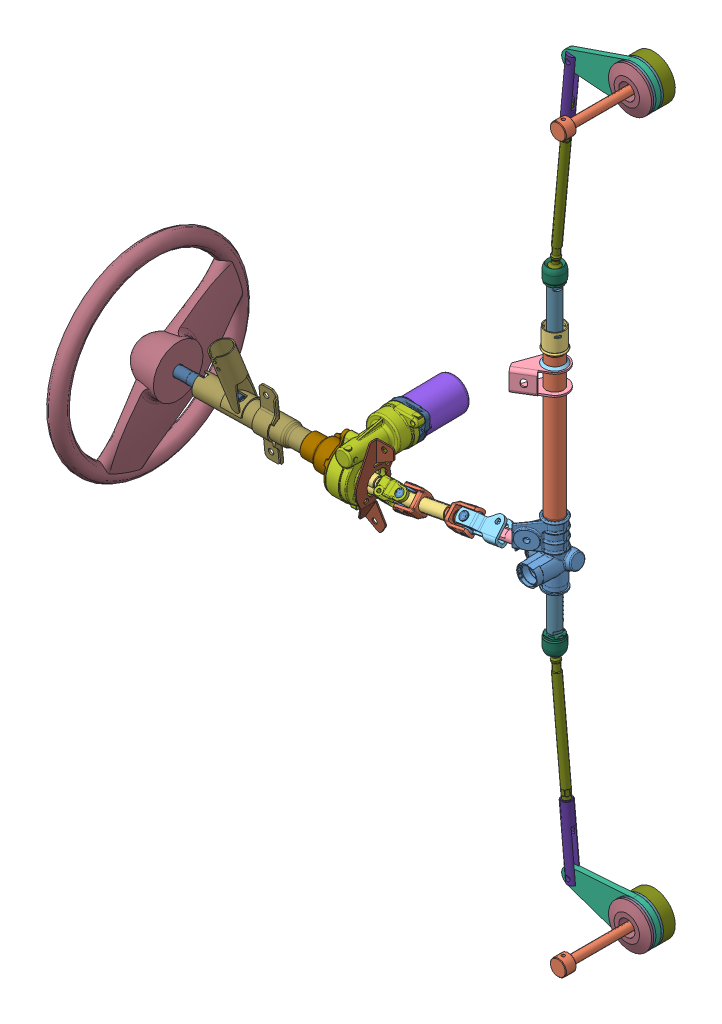
SolidWorks assembly ensemble_dae, configuration Défaut. Lengths in mm.
Overall size (1007.62 1491.77 531.21).
82 component instances, 42 part files, 27 mates.
Components (placement in the parent):
- ensemble_carter-1: ensemble_carter [Défaut] at (126.6085 40.308 0) size (890.36 1491.77 343.25)
  - ensemble_carter_cremaillere-1: ensemble_carter_cremaillere [Défaut] x (0 1 0) z (0.523604 0 0.851962) size (421.75 116.85 117.42)
    - boitier_pignon-1: boitier_pignon [Défaut] at (-210 0 0) x (1 0 0) z (0 0.523604 0.851962) size (118 84.29 86.02)
    - tube_crémaillère-1: tube_crémaillère [Défaut] at (-128 0 0) x (1 0 0) z (0 0.056204 0.998419) size (305.5 35 35)
    - embout_cremaillere-1: embout_cremaillere [Défaut] at (169.0543 0 0) x (1 0 0) z (0 0.056204 0.998419) size (37.25 39.5 39.5)
    - patte_cremaillere-1: patte_cremaillere [Défaut] at (132 -23 27) x (1 0 0) z (0 1 0) size (40.02 51.5 78)
    - bead2-2: bead2 [Défaut] at origin size (4.91 42.26 42.11)
    - bead3-1: bead3 [Défaut] at origin size (4.91 42.26 42.11)
  - ensemble_carter_assistance-1: ensemble_carter_assistance [Défaut] at (-371.6873 -175.5297 -87.7187) x (0.999846 0 -0.017523) z (0.017523 0 0.999846) size (350.5 192.4 245.84)
    - carter_réducteur-1: carter_réducteur [Défaut] at origin size (86 132.9 120)
    - boitier_moteur-1: boitier_moteur [Défaut] at (0.008 -0.4901 -13.5) x (0.999849 0.017398 0) z (0 0 1) size (82.29 66 97)
    - carter_capteur-1: carter_capteur [Défaut] at (-24 -42 76) x (1 0 0) z (0 0.868796 -0.49517) size (86 83.51 98.87)
    - flasque_moteur-1: flasque_moteur [Défaut] at (-0.0002 0.0008 -11) x (1 -0.000004 0) z (0 0 1) size (86 66.52 24)
    - tole_pliée-1: tole_pliée [Défaut] at (27.5612 -42 76) x (0 -1 0) z (0 0 1) size (146.94 53.66 68.51)
    - boitier_tole-1: boitier_tole [Défaut] at (-178.9434 -42 76) x (0 0.995099 0.098888) z (-1 0 0) size (176.09 56.57 208)
  - limiteur_pivot-1: limiteur_pivot [Défaut] at (162.0108 682.0108 -71.6689) x (0 0 -1) z (0.707107 -0.707107 0) size (182 104.49 104.49)
    - moyeu_limiteur-1: moyeu_limiteur [Défaut] at (-80.1689 -14.1574 0) size (54 80 80)
    - rondelle_friction-1: rondelle_friction [Défaut] at (-64.1689 -14.1574 0) x (0 -0.924225 -0.381849) z (1 0 0) size (80 80 4)
    - rondelle_friction-2: rondelle_friction [Défaut] at (-78.1689 -14.1574 0) x (0 0 1) z (-1 0 0) size (80 80 4)
    - palier_limiteur-1: palier_limiteur [Défaut] at (-79.1689 -14.1574 0) size (16 50 50)
    - plateau_presseur-1: plateau_presseur [Défaut] at (-62.1689 -14.1574 0) size (22 80 80)
    - rondelle_belleville-1: rondelle_belleville [Défaut] at (-55.0689 -14.1574 0) x (0 -1 0) z (0 0 1) size (70 3.07 70)
    - rondelle_belleville-2: rondelle_belleville [Défaut] at (-55.0689 -14.1574 0) x (0 1 0) z (0 0 1) size (70 3.07 70)
    - rondelle_frein-1: rondelle_frein [Défaut] at (-51.9989 -14.1574 0) size (4 70 70)
    - ecrou_limiteur-1: ecrou_limiteur [Défaut] at (-39.9989 -14.1574 0) x (-1 0 0) z (0 -0.924225 -0.381849) size (8 70 70)
    - capteur_pivot-1: capteur_pivot [Défaut] at (-38.1689 -14.1574 0) x (0 0.707107 -0.707107) z (0 -0.707107 -0.707107) size (30 180 30)
  - limiteur_pivot-2: limiteur_pivot [Défaut] at (162.0108 -661.9892 -71.6689) x (0 0 -1) z (0.707107 -0.707107 0) size (182 104.49 104.49)
    - moyeu_limiteur-1: moyeu_limiteur [Défaut] at (-80.1689 -14.1574 0) size (54 80 80)
    - rondelle_friction-1: rondelle_friction [Défaut] at (-64.1689 -14.1574 0) x (0 -0.924225 -0.381849) z (1 0 0) size (80 80 4)
    - rondelle_friction-2: rondelle_friction [Défaut] at (-78.1689 -14.1574 0) x (0 0 1) z (-1 0 0) size (80 80 4)
    - palier_limiteur-1: palier_limiteur [Défaut] at (-79.1689 -14.1574 0) size (16 50 50)
    - plateau_presseur-1: plateau_presseur [Défaut] at (-62.1689 -14.1574 0) size (22 80 80)
    - rondelle_belleville-1: rondelle_belleville [Défaut] at (-55.0689 -14.1574 0) x (0 -1 0) z (0 0 1) size (70 3.07 70)
    - rondelle_belleville-2: rondelle_belleville [Défaut] at (-55.0689 -14.1574 0) x (0 1 0) z (0 0 1) size (70 3.07 70)
    - rondelle_frein-1: rondelle_frein [Défaut] at (-51.9989 -14.1574 0) size (4 70 70)
    - ecrou_limiteur-1: ecrou_limiteur [Défaut] at (-39.9989 -14.1574 0) x (-1 0 0) z (0 -0.924225 -0.381849) size (8 70 70)
    - capteur_pivot-1: capteur_pivot [Défaut] at (-38.1689 -14.1574 0) x (0 0.707107 -0.707107) z (0 -0.707107 -0.707107) size (30 180 30)
- ensemble_recepteur-1: ensemble_recepteur [Défaut] at (-300.2029 -311.4891 -138.9484) x (-0.999846 0 0.017523) z (-0.012674 0.690542 -0.723182) size (124 97.96 97.96)
  - ensemble_roue-1: ensemble_roue [Défaut] at (-32.6877 82.9298 0) size (91 97.96 97.96)
    - arbre_roue-1: arbre_roue [Défaut] at (-15.5303 102.7038 0) size (88 32 32)
    - creneaux_roue-1: creneaux_roue [Défaut] at (-0.5303 102.7038 0) size (10 31 31)
    - moyeu_roue-1: moyeu_roue [Défaut] at (-27.5303 102.7038 0) x (1 0 0) z (0 -0.027331 0.999626) size (12 62 62)
    - roue-1: roue [Défaut] at (-26.5303 102.7038 0) x (-1 0 0) z (0 0.924225 -0.381849) size (10 75 75)
  - fourche_cardan-1: fourche_cardan [Défaut] at (-93.2179 185.75 -1.9966) x (0 0.998307 0.058156) z (0 -0.058156 0.998307) size (42.34 54.79 32.31)
- ensemble_volant-1: ensemble_volant [Défaut] at (-165.4037 -293.1598 -131.9435) x (-0.999846 0 0.017523) z (-0.012674 0.690542 -0.723182) size (466.36 370 370)
  - barre_de_torsion-1: barre_de_torsion [Défaut] at (165.9378 165.9087 -5.8829) x (1 0 0) z (0 -1 0) size (145 8 8)
  - creneaux_colonne-1: creneaux_colonne [Défaut] at (117.8546 165.9087 -5.8829) x (-1 0 0) z (0 0.979628 -0.200818) size (30 31 31)
  - arbre_trans_ext-1: arbre_trans_ext [Défaut] at (443.3272 165.9087 -5.8829) x (-1 0 0) z (0 0.159988 0.987119) size (204 30 30)
  - arbre_trans_int-1: arbre_trans_int [Défaut] at (179.1633 165.9087 -5.8829) x (1 0 0) z (0 0.159988 0.987119) size (115 17 17)
  - moyeu_de_capteur-1: moyeu_de_capteur [Défaut] at (101.983 165.9087 -5.8829) x (-1 0 0) z (0 0.299586 0.954069) size (88 28 28)
  - volant-1: volant [Défaut] at (470.1285 165.9087 -5.8829) size (73.29 370 370)
- ensemble_cremaillere-1: ensemble_cremaillere [Défaut] at (126.6085 -91.4682 -18.936) x (0 1 0) z (-1 0 0) size (623.5 47.69 47.69)
  - Crémaillère-1: Crémaillère [Défaut] at (131.7762 -18.936 0) size (560 22 22)
  - cremaillere_embout-1: cremaillere_embout [Défaut] at (-170.2238 -18.936 0) x (1 0 0) z (0 -0.229093 0.973405) size (45.75 34 34)
  - cremaillere_embout-2: cremaillere_embout [Défaut] at (433.7762 -18.936 0) x (-1 0 0) z (0 -0.791815 -0.610761) size (45.75 34 34)
- biellette_1-1: biellette_1 [Défaut] at (89.6983 343.1262 40.7275) x (0.092743 0.99569 0) z (-0.99569 0.092743 0) size (375.97 24 24)
  - Biellette-1: Biellette [Défaut] at (2.6085 40.7275 -36.827) size (290 24 24)
  - embout_rotule-1: embout_rotule [Défaut] at (238.5785 40.7275 -36.827) size (130 20 20)
- ensemble_croisillon-1: ensemble_croisillon [Défaut] at (-178.3174 -280.3328 -98.2422) x (0.011342 0.762228 0.64721) z (-0.124553 0.643287 -0.755426) size (40.4 20.18 40.4)
  - croisillon-1: croisillon [Défaut] at (133.8433 15.1586 0) size (36 20 36)
  - roult_aiguilles-1: roult_aiguilles [Défaut] at (113.8433 15.1586 0) x (1 0 0) z (0 -0.005579 0.999984) size (10 15 15)
  - roult_aiguilles-2: roult_aiguilles [Défaut] at (153.8433 15.1586 0) x (-1 0 0) z (0 -0.983447 0.181195) size (10 15 15)
  - roult_aiguilles-3: roult_aiguilles [Défaut] at (133.8433 15.1586 -20) x (0 0 1) z (-0.454157 0.890922 0) size (10 15 15)
  - roult_aiguilles-4: roult_aiguilles [Défaut] at (133.8433 15.1586 20) x (0 0 -1) z (0.994379 0.105875 0) size (10 15 15)
- ensemble_transmission-2: ensemble_transmission [Défaut] at (-59.2719 -157.5062 -13.2763) x (0.124553 -0.643287 0.755426) z (-0.142032 0.741954 0.655233) size (42 202 30.26)
  - fourche_cardan_3-1: fourche_cardan_3 [Défaut] at origin size (42 79 30.26)
  - arbre_transmission-1: arbre_transmission [Défaut] at origin size (22 150 22)
- ensemble_pignon-1: ensemble_pignon [Défaut] at (190.9556 -108.5326 -18.4657) x (0.984808 0.173648 0) z (-0.131186 0.743994 0.655182) size (206.84 48.43 47.04)
  - pignon-1: pignon [Défaut] at (-214.1756 -7.2348 0) size (171 18.5 18.5)
  - fourche_cardan_4-1: fourche_cardan_4 [Défaut] at (-173.9126 -25.7617 0.3119) x (-0.000233 -0.173648 -0.984808) z (-0.999999 0.001339 0) size (40.37 41.95 76.1)
- ensemble_croisillon-2: ensemble_croisillon [Défaut] at (-43.2639 -51.5992 74.2701) x (0.131186 -0.743994 -0.655182) z (-0.124553 0.643287 -0.755426) size (40.4 20.18 40.4)
  - croisillon-1: croisillon [Défaut] at (133.8433 15.1586 0) size (36 20 36)
  - roult_aiguilles-1: roult_aiguilles [Défaut] at (113.8433 15.1586 0) x (1 0 0) z (0 -0.005579 0.999984) size (10 15 15)
  - roult_aiguilles-2: roult_aiguilles [Défaut] at (153.8433 15.1586 0) x (-1 0 0) z (0 -0.983447 0.181195) size (10 15 15)
  - roult_aiguilles-3: roult_aiguilles [Défaut] at (133.8433 15.1586 -20) x (0 0 1) z (-0.454157 0.890922 0) size (10 15 15)
  - roult_aiguilles-4: roult_aiguilles [Défaut] at (133.8433 15.1586 20) x (0 0 -1) z (0.994379 0.105875 0) size (10 15 15)
- fourche_cardan_3-2: fourche_cardan_3 [Défaut] at (-143.1018 -173.6325 -13.1871) x (-0.124553 0.643287 -0.755426) z (-0.142032 0.741954 0.655233) size (42 79 30.26)
- levier_pivot-1: levier_pivot [Défaut] at (278.6085 -631.692 -0.5) x (-0.991553 0.129702 0) z (0 0 1) size (176 80 10)
- levier_pivot-2: levier_pivot [Défaut] at (278.6085 712.308 -0.5) x (-0.991553 -0.129702 0) z (0 0 1) size (176 80 10)
- biellette_1-2: biellette_1 [Défaut] at (163.0349 -255.6793 40.7275) x (0.092743 -0.99569 0) z (0.99569 0.092743 0) size (375.97 24 24)
  - Biellette-1: Biellette [Défaut] at (2.6085 40.7275 -36.827) size (290 24 24)
  - embout_rotule-1: embout_rotule [Défaut] at (238.5785 40.7275 -36.827) size (130 20 20)
Mates (geometry in assembly coordinates):
- Coaxialité crémaillère corps: concentric anti-aligned: cylinder of ensemble_carter-1/ensemble_carter_cremaillere-1/tube_crémaillère-1 through (126.6085 -87.692 0) axis (0 -1 0) radius 16; cylinder of ensemble_cremaillere-1/Crémaillère-1 through (126.6085 341.308 0) axis (0 1 0) radius 11
- Parallèle orientation angulaire crémaillère corps: parallel anti-aligned: plane of ensemble_carter-1/ensemble_carter_cremaillere-1/boitier_pignon-1 through (126.6085 -169.692 -10) normal (0 0 1); plane of ensemble_cremaillere-1/Crémaillère-1 through (139.1085 -222.2361 -8) normal (0 0 -1)
- Coaxialité croisillon supérieur / récepteur: concentric anti-aligned: cylinder of ensemble_recepteur-1/fourche_cardan-1 through (-161.5196 -161.0851 0.5344) axis (-0.011342 -0.762228 -0.64721) radius 7; cylinder of ensemble_croisillon-1/roult_aiguilles-2 through (-161.5328 -161.9771 -0.223) axis (0.011342 0.762228 0.64721) radius 7.5
- Position axiale croisillon supérieur / récepteur: coincident aligned: plane of ensemble_recepteur-1/fourche_cardan-1; plane of ensemble_croisillon-1/croisillon-1
- Coaxialité pignon / corps: concentric aligned: cylinder of ensemble_carter-1/ensemble_carter_cremaillere-1/boitier_pignon-1 through (73.6576 -134.0287 -13) axis (-0.984808 -0.173648 0) radius 16; cylinder of ensemble_pignon-1/pignon-1 through (-19.143 -150.3919 -13) axis (-0.984808 -0.173648 0) radius 9
- distance arrêt en translation pignon / corps: distance = 8 mm anti-aligned: plane of ensemble_carter-1/ensemble_carter_cremaillere-1/boitier_pignon-1 through (77.3681 -133.3744 -32.5) normal (-0.984808 -0.173648 0); plane of ensemble_pignon-1/pignon-1 through (68.4373 -128.7952 -19.9881) normal (0.984808 0.173648 0)
- Coaxialité croisillon inférieur / pignon: concentric aligned: cylinder of ensemble_pignon-1/fourche_cardan_4-1 through (-43.0267 -140.2341 -1.2467) axis (0.131186 -0.743994 -0.655182) radius 7.5; cylinder of ensemble_croisillon-2/roult_aiguilles-2 through (-37.9903 -168.7969 -26.3998) axis (0.131186 -0.743994 -0.655182) radius 7.5
- Position axiale croisillon inférieur / pignon: coincident anti-aligned: plane of ensemble_pignon-1 through (190.9556 -108.5326 -18.4657) normal (-0.131186 0.743994 0.655182); plane of ensemble_croisillon-2/croisillon-1
- Coaxialité croisillon supérieur / inter: concentric anti-aligned: cylinder of ensemble_croisillon-1/roult_aiguilles-3 through (-159.2686 -190.0874 1.9413) axis (0.124553 -0.643287 0.755426) radius 7.5; cylinder of fourche_cardan_3-2 through (-158.6459 -193.3039 5.7184) axis (-0.124553 0.643287 -0.755426) radius 7.5
- Position axiale croisillon supérieur / inter: coincident aligned: plane of ensemble_croisillon-1/croisillon-1 through (-161.7597 -177.2217 -13.1672) normal (-0.124553 0.643287 -0.755426); plane of fourche_cardan_3-2
- Coaxialité croisillon inférieur / inter: concentric aligned: cylinder of ensemble_transmission-2/fourche_cardan_3-1 through (-43.7278 -137.8348 -32.1818) axis (0.124553 -0.643287 0.755426) radius 7.5; cylinder of ensemble_croisillon-2/roult_aiguilles-3 through (-38.123 -166.7827 1.8123) axis (0.124553 -0.643287 0.755426) radius 7.5
- Position axiale croisillon inférieur / inter: coincident anti-aligned: plane of ensemble_transmission-2/fourche_cardan_3-1; plane of ensemble_croisillon-2/croisillon-1 through (-40.614 -153.917 -13.2962) normal (-0.124553 0.643287 -0.755426)
- Coaxialité arbre de transmission / cardan inférieur: concentric anti-aligned: cylinder of ensemble_transmission-2/fourche_cardan_3-1 through (-59.2719 -157.5062 -13.2763) axis (0.981995 0.188906 -0.001045) radius 9; cylinder of fourche_cardan_3-2 through (-143.1018 -173.6325 -13.1871) axis (-0.981995 -0.188906 0.001045) radius 9
- Position angulaire arbre de transmission / cardan inférieur: parallel aligned: plane of ensemble_transmission-2/fourche_cardan_3-1 through (-59.2719 -157.5062 -13.2763) normal (-0.142032 0.741954 0.655233); plane of fourche_cardan_3-2 through (-143.1018 -173.6325 -13.1871) normal (-0.142032 0.741954 0.655233)
- Coaxialité récpteur / carter: concentric anti-aligned: cylinder of ensemble_carter-1/ensemble_carter_assistance-1/carter_réducteur-1 through (-197.2542 -177.2217 -12.5452) axis (0.999846 0 -0.017523) radius 21; cylinder of ensemble_recepteur-1/ensemble_roue-1/arbre_roue-1 through (-287.7403 -177.2217 -10.9594) axis (-0.999846 0 0.017523) radius 10
- Position axiale récepteur / carter: distance = 0 mm aligned: plane of ensemble_carter-1/ensemble_carter_assistance-1/carter_réducteur-1 through (-229.7493 -156.2217 -11.9757) normal (0.999846 0 -0.017523); plane of ensemble_recepteur-1/ensemble_roue-1/arbre_roue-1 through (-229.6162 -169.2655 -4.3809) normal (0.999846 0 -0.017523)
- Coaxialité volant / carter: concentric anti-aligned: cylinder of ensemble_carter-1/ensemble_carter_assistance-1/boitier_tole-1 through (-422.663 -177.2217 -8.5948) axis (0.999846 0 -0.017523) radius 18.5; cylinder of ensemble_volant-1/arbre_trans_ext-1 through (-614.5795 -177.2217 -5.2315) axis (-0.999846 0 0.017523) radius 10
- coaxialité goupille barre de torsion recepteur: concentric aligned: cylinder of ensemble_recepteur-1/ensemble_roue-1/arbre_roue-1 through (-189.5526 -188.2704 -1.1057) axis (-0.012674 0.690542 -0.723182) radius 2; cylinder of ensemble_volant-1/barre_de_torsion-1 through (-189.7047 -179.9839 -9.7839) axis (-0.012674 0.690542 -0.723182) radius 2
- Coïncidente2: coincident anti-aligned: plane of ensemble_carter-1/limiteur_pivot-1/rondelle_friction-2 through (278.6085 712.308 4.5) normal (0 0 -1); plane of levier_pivot-2 through (278.6085 712.308 4.5) normal (0 0 1)
- Coaxial4: concentric anti-aligned: cylinder of ensemble_carter-1/limiteur_pivot-1/palier_limiteur-1 through (278.6085 712.308 7.5) axis (0 0 1) radius 25; cylinder of levier_pivot-2 through (278.6085 712.308 4.5) axis (0 0 -1) radius 22.5
- Coïncidente3: coincident anti-aligned: plane of ensemble_carter-1/limiteur_pivot-2/rondelle_friction-2 through (278.6085 -631.692 4.5) normal (0 0 -1); plane of levier_pivot-1 through (278.6085 -631.692 4.5) normal (0 0 1)
- Coaxial5: concentric anti-aligned: cylinder of ensemble_carter-1/limiteur_pivot-2/palier_limiteur-1 through (278.6085 -631.692 7.5) axis (0 0 1) radius 25; cylinder of levier_pivot-1 through (278.6085 -631.692 4.5) axis (0 0 -1) radius 22.5
- Coïncidente6: coincident: point of ensemble_cremaillere-1/cremaillere_embout-2; point of biellette_1-1/Biellette-1
- Coïncidente7: coincident: point of ensemble_cremaillere-1/cremaillere_embout-1; point of biellette_1-2/Biellette-1
- Coïncidente8: coincident: point of ensemble_carter-1; point of ensemble_cremaillere-1/Crémaillère-1
- Coaxiale1: concentric aligned: cylinder of levier_pivot-1 through (159.6221 -616.1278 4.5) axis (0 0 -1) radius 6; cylinder of biellette_1-2/embout_rotule-1 through (159.6221 -616.1278 10) axis (0 0 -1) radius 4.5
- Coaxiale2: concentric aligned: cylinder of biellette_1-1/embout_rotule-1 through (159.6221 696.7438 10) axis (0 0 -1) radius 4.5; cylinder of levier_pivot-2 through (159.6221 696.7438 4.5) axis (0 0 -1) radius 6
